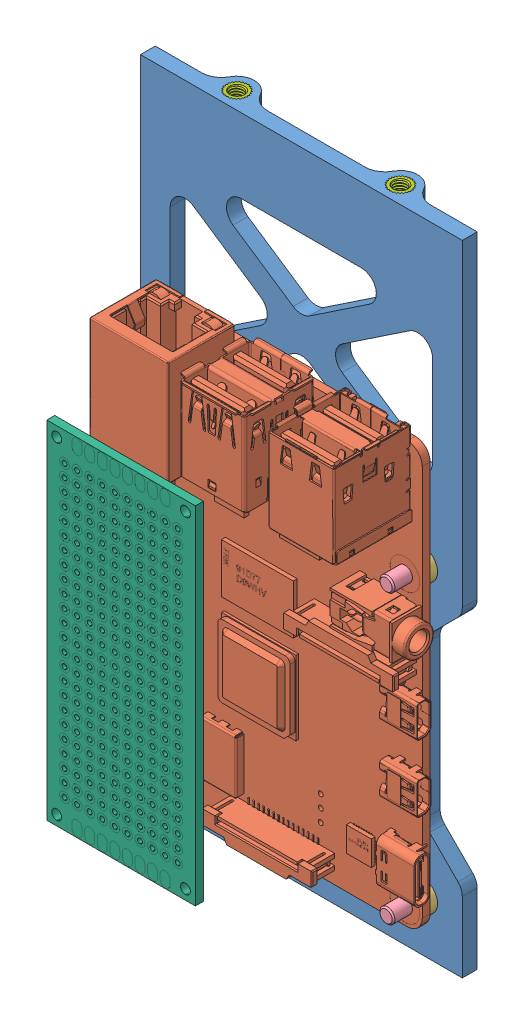
SolidWorks assembly ASM-level-raspberry-pi, configuration По умолчанию. Lengths in mm.
Overall size (65 129.01 28.74).
17 component instances, 7 part files, 21 mates.
Components (placement in the parent):
- level-2-1: level-2 [По умолчанию] at origin size (65 129 7)
- Raspberry Pi 4 Model B-1: Raspberry Pi 4 Model B [По умолчанию] at (0 -15 5.79) x (0 1 0) z (1 0 0) size (88.99 19.91 58.4)
- 3-6-3-1: 3-6-3 [По умолчанию] at (-24.5 -54 3) size (6 6 2)
- 3-6-3-2: 3-6-3 [По умолчанию] at (-24.5 4 3) size (6 6 2)
- 3-6-3-3: 3-6-3 [По умолчанию] at (24.5 4 3) size (6 6 2)
- 3-6-3-4: 3-6-3 [По умолчанию] at (24.5 -54 3) x (0.98212 -0.188257 0) z (0 0 1) size (6 6 2)
- socket countersunk head screw_iso-1: socket countersunk head screw_iso [ISO 10642 - M3 x 10 - 10N] at (24.5 -54 0.39) x (0 0 1) z (-0.999977 -0.006797 0) size (10 5.54 5.54)
- socket countersunk head screw_iso-2: socket countersunk head screw_iso [ISO 10642 - M3 x 10 - 10N] at (24.5 4 0.39) x (0 0 1) z (-0.999917 -0.012873 0) size (10 5.54 5.54)
- socket countersunk head screw_iso-3: socket countersunk head screw_iso [ISO 10642 - M3 x 10 - 10N] at (-24.5 4 0.39) x (0 0 1) z (-0.999928 -0.012001 0) size (10 5.54 5.54)
- socket countersunk head screw_iso-4: socket countersunk head screw_iso [ISO 10642 - M3 x 10 - 10N] at (-24.5 -54 0.39) x (0 0 1) z (-1 -0.000767 0) size (10 5.54 5.54)
- ASM-shild-raspberry-1: ASM-shild-raspberry [По умолчанию] at (-22.18 0.88 25.14) x (1 0 0) z (0 1 0) size (30 10.65 70)
  - 40 pin connector header smt v3.step-1: 40 pin connector header smt v3.step [По умолчанию] at origin size (5.18 10.05 51.4)
  - Breadboard 30 х 70 mm.step-1: Breadboard 30 х 70 mm.step [По умолчанию] at (7.5097 0.4 -23.0097) size (30 1.65 70)
- M3 insert nut.step-1: M3 insert nut.step [По умолчанию] at (16.5 -61.4 -0.5) x (1 0 0) z (0 -1 0) size (4.49 4.48 6.21)
- M3 insert nut.step-2: M3 insert nut.step [По умолчанию] at (-16.5 -61.4 -0.5) x (1 0 0) z (0 -1 0) size (4.49 4.48 6.21)
- M3 insert nut.step-3: M3 insert nut.step [По умолчанию] at (16.5 61.4001 -0.5) x (1 0 0) z (0 -1 0) size (4.49 4.48 6.21)
- M3 insert nut.step-4: M3 insert nut.step [По умолчанию] at (-16.5 61.4001 -0.5) x (1 0 0) z (0 -1 0) size (4.49 4.48 6.21)
Mates (geometry in assembly coordinates):
- Концентричный1: concentric anti-aligned: cylinder of level-2-1 through (-24.5 -54 -7) axis (0 0 1) radius 1.75; cylinder of 3-6-3-1 through (-24.5 -54 5) axis (0 0 -1) radius 1.75
- Концентричный2: concentric anti-aligned: cylinder of level-2-1 through (-24.5 4 -7) axis (0 0 1) radius 1.75; cylinder of 3-6-3-2 through (-24.5 4 5) axis (0 0 -1) radius 1.75
- Концентричный3: concentric anti-aligned: cylinder of level-2-1 through (24.5 4 -7) axis (0 0 1) radius 1.75; cylinder of 3-6-3-3 through (24.5 4 5) axis (0 0 -1) radius 1.75
- Концентричный4: concentric anti-aligned: cylinder of level-2-1 through (24.5 -54 -7) axis (0 0 1) radius 1.75; cylinder of 3-6-3-4 through (24.5 -54 5) axis (0 0 -1) radius 1.75
- Совпадение1: coincident aligned: plane of 3-6-3-1 through (-24.5 -54 5) normal (0 0 1); plane of 3-6-3-4 through (24.5 -54 5) normal (0 0 1)
- Совпадение2: coincident aligned: plane of 3-6-3-2 through (-24.5 4 5) normal (0 0 1); plane of 3-6-3-3 through (24.5 4 5) normal (0 0 1)
- Совпадение3: coincident aligned: plane of 3-6-3-3 through (24.5 4 5) normal (0 0 1); plane of 3-6-3-4 through (24.5 -54 5) normal (0 0 1)
- Совпадение4: coincident anti-aligned: plane of level-2-1 through (0 0 3) normal (0 0 1); plane of 3-6-3-4 through (24.5 -54 3) normal (0 0 -1)
- Концентричный5: concentric anti-aligned: cylinder of Raspberry Pi 4 Model B-1 through (24.5 -54 6.59) axis (0 0 1) radius 1.35; cylinder of 3-6-3-4 through (24.5 -54 5) axis (0 0 -1) radius 1.75
- Совпадение5: coincident anti-aligned: plane of Raspberry Pi 4 Model B-1 through (24.5 -54 5) normal (0 0 -1); plane of 3-6-3-4 through (24.5 -54 5) normal (0 0 1)
- Совпадение6: coincident aligned: cone of level-2-1 through (24.5 -54 0) axis (0 0 1); cone of socket countersunk head screw_iso-1 through (24.5 -54 0.98) axis (0 0 1)
- Совпадение7: coincident aligned: cone of level-2-1 through (24.5 4 0) axis (0 0 1); cone of socket countersunk head screw_iso-2 through (24.5 4 0.98) axis (0 0 1)
- Совпадение8: coincident aligned: cone of level-2-1 through (-24.5 4 0) axis (0 0 1); cone of socket countersunk head screw_iso-3 through (-24.5 4 0.98) axis (0 0 1)
- Совпадение9: coincident aligned: cone of level-2-1 through (-24.5 -54 0) axis (0 0 1); cone of socket countersunk head screw_iso-4 through (-24.5 -54 0.98) axis (0 0 1)
- Совпадение10: coincident anti-aligned: plane of Raspberry Pi 4 Model B-1 through (-23.55 -49.45 14.89) normal (0 -1 0); plane of ASM-shild-raspberry-1/40 pin connector header smt v3.step-1 through (-23.91 -49.45 14.09) normal (0 1 0)
- Совпадение11: coincident anti-aligned: plane of Raspberry Pi 4 Model B-1 through (-22.91 -49.45 14.89) normal (1 0 0); plane of ASM-shild-raspberry-1/40 pin connector header smt v3.step-1 through (-22.91 -49.45 14.09) normal (-1 0 0)
- Расстояние1: distance = 5 mm anti-aligned: plane of Raspberry Pi 4 Model B-1 through (-25.77 -49.13 9.09) normal (0 0 1); plane of ASM-shild-raspberry-1/40 pin connector header smt v3.step-1 through (-24.68 -24.82 14.09) normal (0 0 -1)
- Концентричный6: concentric anti-aligned: cylinder of level-2-1 through (-16.5 -58.5 -0.5) axis (0 -1 0) radius 2; cylinder of M3 insert nut.step-2 through (-16.5 -64.5 -0.5) axis (0 1 0) radius 2
- Совпадение12: coincident aligned: plane of level-2-1 through (0 -64.5 3) normal (0 -1 0); plane of M3 insert nut.step-2 through (-16.5 -64.5 -0.5) normal (0 -1 0)
- Концентричный7: concentric anti-aligned: cylinder of level-2-1 through (16.5 -58.5 -0.5) axis (0 -1 0) radius 2; cylinder of M3 insert nut.step-1 through (16.5 -64.5 -0.5) axis (0 1 0) radius 2
- Совпадение13: coincident aligned: plane of level-2-1 through (0 -64.5 3) normal (0 -1 0); plane of M3 insert nut.step-1 through (16.5 -64.5 -0.5) normal (0 -1 0)
